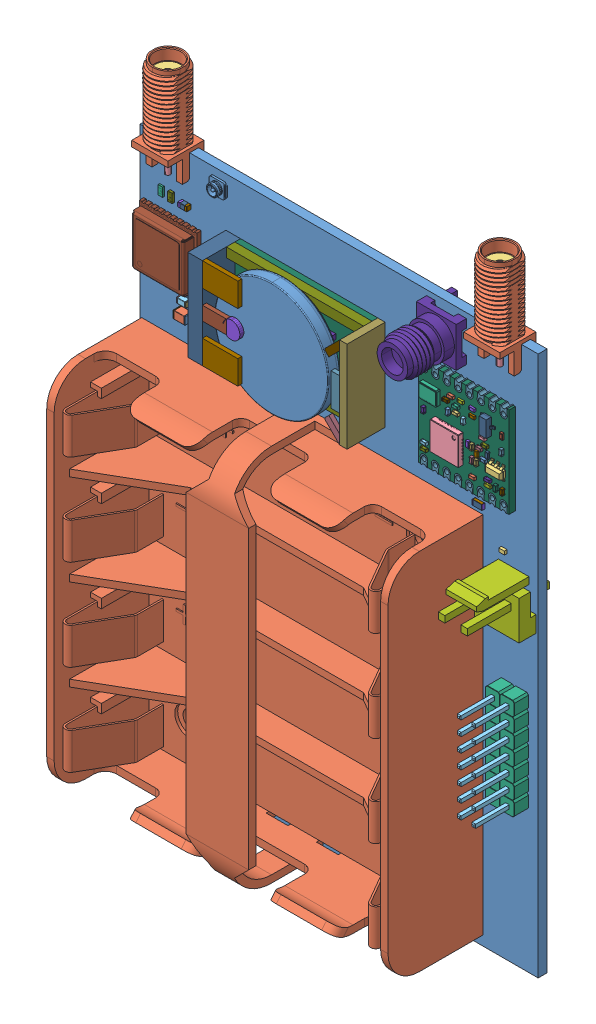
SolidWorks assembly Печатная плата Peggy Tracker, configuration Default. Lengths in mm.
Overall size (70 108.1 20.64).
358 component instances, 132 part files, 0 mates.
Components (placement in the parent):
- Печатная плата Peggy Tracker(2)^Печатная плата Peggy Tracker-1: Печатная плата Peggy Tracker(2)^Печатная плата Peggy Tracker [Default] at origin size (70 108.1 20.64) (virtual)
  - Board^Печатная плата Peggy Tracker(2)_Печатная плата Peggy Tracker-1: Board^Печатная плата Peggy Tracker(2)_Печатная плата Peggy Tracker [Default] at origin size (70 95 1.56) (virtual)
    - Open CASCADE STEP translator 6.8 1.1.1^Board_Печатная плата Peggy Tracker(2)_Печатная плата Peggy Tracker-1: Open CASCADE STEP translator 6.8 1.1.1^Board_Печатная плата Peggy Tracker(2)_Печатная плата Peggy Tracker [По умолчанию] at (0 0 -1.5596) size (70 95 1.56) (virtual)
  - XW4^Печатная плата Peggy Tracker(2)_Печатная плата Peggy Tracker-1: XW4^Печатная плата Peggy Tracker(2)_Печатная плата Peggy Tracker [Default] at origin size (6.87 17.48 6.87) (virtual)
    - SMA_female_edge_6.5x6.5^XW4_Печатная плата Peggy Tracker(2)_Печатная плата Peggy Tracker-1: SMA_female_edge_6.5x6.5^XW4_Печатная плата Peggy Tracker(2)_Печатная плата Peggy Tracker [Default] at (63.8984 92.1251 0.2) x (-1 0 0) z (0 0 1) size (6.87 17.48 6.87) (virtual)
      - SMA_female_edge_6.5x6^SMA_female_edge_6.5x6.5_XW4_Печатная плата Peggy Tracker(2)_Печатная плата Peggy Tracker-1: SMA_female_edge_6.5x6^SMA_female_edge_6.5x6.5_XW4_Печатная плата Peggy Tracker(2)_Печатная плата Peggy Tracker [Default] at origin size (6.87 17.48 6.87) (virtual)
        - ^SMA_female_edge_6.5x6_SMA_female_edge_6.5x6.5_XW4_Печатная плата Peggy Tracker(2)_Печатная плата Peggy Tracker-1: ^SMA_female_edge_6.5x6_SMA_female_edge_6.5x6.5_XW4_Печатная плата Peggy Tracker(2)_Печатная плата Peggy Tracker [По умолчанию] at (0 -4 0.45) x (0 0 1) z (0 -1 0) size (6.87 6.87 17.29) (virtual)
        - Copy (2) of ^SMA_female_edge_6.5x6_SMA_female_edge_6.5x6.5_XW4_Печатная плата Peggy Tracker(2)_Печатная плата Peggy Tracker-1: Copy (2) of ^SMA_female_edge_6.5x6_SMA_female_edge_6.5x6.5_XW4_Печатная плата Peggy Tracker(2)_Печатная плата Peggy Tracker [По умолчанию] at (0 -4 0.45) x (0 0 1) z (0 -1 0) size (4.25 4.25 11.54) (virtual)
        - Copy (3) of ^SMA_female_edge_6.5x6_SMA_female_edge_6.5x6.5_XW4_Печатная плата Peggy Tracker(2)_Печатная плата Peggy Tracker-1: Copy (3) of ^SMA_female_edge_6.5x6_SMA_female_edge_6.5x6.5_XW4_Печатная плата Peggy Tracker(2)_Печатная плата Peggy Tracker [По умолчанию] at (0 -4 0.45) x (0 0 1) z (0 -1 0) size (1.27 1.27 15.54) (virtual)
  - C21^Печатная плата Peggy Tracker(2)_Печатная плата Peggy Tracker-1: C21^Печатная плата Peggy Tracker(2)_Печатная плата Peggy Tracker [Default] at origin size (1.6 0.8 0.3) (virtual)
    - SW3dPS-0603_SMD_Capacitor^C21_Печатная плата Peggy Tracker(2)_Печатная плата Peggy Tracker-1: SW3dPS-0603_SMD_Capacitor^C21_Печатная плата Peggy Tracker(2)_Печатная плата Peggy Tracker [По умолчанию] at (25.6001 31.0999 -1.5596) x (1 0 0) z (0 1 0) size (1.6 0.3 0.8) (virtual)
  - C20^Печатная плата Peggy Tracker(2)_Печатная плата Peggy Tracker-1: C20^Печатная плата Peggy Tracker(2)_Печатная плата Peggy Tracker [Default] at origin size (3.2 1.6 1) (virtual)
    - SW3dPS-1206_SMD_Capacitor^C20_Печатная плата Peggy Tracker(2)_Печатная плата Peggy Tracker-1: SW3dPS-1206_SMD_Capacitor^C20_Печатная плата Peggy Tracker(2)_Печатная плата Peggy Tracker [По умолчанию] at (30.5 25 -1.5596) x (1 0 0) z (0 1 0) size (3.2 1 1.6) (virtual)
  - C19^Печатная плата Peggy Tracker(2)_Печатная плата Peggy Tracker-1: C19^Печатная плата Peggy Tracker(2)_Печатная плата Peggy Tracker [Default] at origin size (1.6 0.8 0.3) (virtual)
    - SW3dPS-0603_SMD_Capacitor^C19_Печатная плата Peggy Tracker(2)_Печатная плата Peggy Tracker-1: SW3dPS-0603_SMD_Capacitor^C19_Печатная плата Peggy Tracker(2)_Печатная плата Peggy Tracker [По умолчанию] at (27.9999 46.9001 -1.5596) x (-1 0 0) z (0 -1 0) size (1.6 0.3 0.8) (virtual)
  - C18^Печатная плата Peggy Tracker(2)_Печатная плата Peggy Tracker-1: C18^Печатная плата Peggy Tracker(2)_Печатная плата Peggy Tracker [Default] at origin size (0.8 1.6 0.3) (virtual)
    - SW3dPS-0603_SMD_Capacitor^C18_Печатная плата Peggy Tracker(2)_Печатная плата Peggy Tracker-1: SW3dPS-0603_SMD_Capacitor^C18_Печатная плата Peggy Tracker(2)_Печатная плата Peggy Tracker [По умолчанию] at (40.0999 43.0999 -1.5596) x (0 -1 0) z (1 0 0) size (1.6 0.3 0.8) (virtual)
  - C17^Печатная плата Peggy Tracker(2)_Печатная плата Peggy Tracker-1: C17^Печатная плата Peggy Tracker(2)_Печатная плата Peggy Tracker [Default] at origin size (0.8 1.6 0.3) (virtual)
    - SW3dPS-0603_SMD_Capacitor^C17_Печатная плата Peggy Tracker(2)_Печатная плата Peggy Tracker-1: SW3dPS-0603_SMD_Capacitor^C17_Печатная плата Peggy Tracker(2)_Печатная плата Peggy Tracker [По умолчанию] at (39.9001 34.9001 -1.5596) x (0 1 0) z (-1 0 0) size (1.6 0.3 0.8) (virtual)
  - C16^Печатная плата Peggy Tracker(2)_Печатная плата Peggy Tracker-1: C16^Печатная плата Peggy Tracker(2)_Печатная плата Peggy Tracker [Default] at origin size (1.6 0.8 0.3) (virtual)
    - SW3dPS-0603_SMD_Capacitor^C16_Печатная плата Peggy Tracker(2)_Печатная плата Peggy Tracker-1: SW3dPS-0603_SMD_Capacitor^C16_Печатная плата Peggy Tracker(2)_Печатная плата Peggy Tracker [По умолчанию] at (22.1999 32.8001 -1.5596) x (-1 0 0) z (0 -1 0) size (1.6 0.3 0.8) (virtual)
  - DD1^Печатная плата Peggy Tracker(2)_Печатная плата Peggy Tracker-1: DD1^Печатная плата Peggy Tracker(2)_Печатная плата Peggy Tracker [Default] at origin size (10.1 9.7 2.7) (virtual)
    - MAX-M8C-0^DD1_Печатная плата Peggy Tracker(2)_Печатная плата Peggy Tracker-1: MAX-M8C-0^DD1_Печатная плата Peggy Tracker(2)_Печатная плата Peggy Tracker [По умолчанию] at (5.7001 79.2999 0) x (0 1 0) z (1 0 0) size (9.7 2.7 10.1) (virtual)
  - ZQ2^Печатная плата Peggy Tracker(2)_Печатная плата Peggy Tracker-1: ZQ2^Печатная плата Peggy Tracker(2)_Печатная плата Peggy Tracker [Default] at origin size (3.22 1.52 0.91) (virtual)
    - User_Library-ABS07^ZQ2_Печатная плата Peggy Tracker(2)_Печатная плата Peggy Tracker-1: User_Library-ABS07^ZQ2_Печатная плата Peggy Tracker(2)_Печатная плата Peggy Tracker [Default] at (18.5999 54.9001 -1.5596) x (-1 0 0) z (0 -1 0) size (3.22 0.91 1.52) (virtual)
      - User_Library-ABS07_ABS07_Body_2^User_Library-ABS07_ZQ2_Печатная плата Peggy Tracker(2)_Печатная плата Peggy Tracker-1: User_Library-ABS07_ABS07_Body_2^User_Library-ABS07_ZQ2_Печатная плата Peggy Tracker(2)_Печатная плата Peggy Tracker [По умолчанию] x (1 0 0) z (0 1 0) size (3.2 1.5 0.85) (virtual)
      - User_Library-ABS07_ABS07_Body2_2^User_Library-ABS07_ZQ2_Печатная плата Peggy Tracker(2)_Печатная плата Peggy Tracker-1: User_Library-ABS07_ABS07_Body2_2^User_Library-ABS07_ZQ2_Печатная плата Peggy Tracker(2)_Печатная плата Peggy Tracker [По умолчанию] x (-1 0 0) z (0 1 0) size (3 1.3 0.05) (virtual)
      - User_Library-ABS07_ABS07_Beschriftung_2^User_Library-ABS07_ZQ2_Печатная плата Peggy Tracker(2)_Печатная плата Peggy Tracker-1: User_Library-ABS07_ABS07_Beschriftung_2^User_Library-ABS07_ZQ2_Печатная плата Peggy Tracker(2)_Печатная плата Peggy Tracker [По умолчанию] x (-1 0 0) z (0 1 0) size (2.05 0.49 0.06) (virtual)
      - User_Library-ABS07_ABS07_Pads_2^User_Library-ABS07_ZQ2_Печатная плата Peggy Tracker(2)_Печатная плата Peggy Tracker-1: User_Library-ABS07_ABS07_Pads_2^User_Library-ABS07_ZQ2_Печатная плата Peggy Tracker(2)_Печатная плата Peggy Tracker [По умолчанию] x (1 0 0) z (0 1 0) size (3.22 1.52 0.25) (virtual)
  - ZQ1^Печатная плата Peggy Tracker(2)_Печатная плата Peggy Tracker-1: ZQ1^Печатная плата Peggy Tracker(2)_Печатная плата Peggy Tracker [Default] at origin size (3.18 5 1.11) (virtual)
    - ABM3B^ZQ1_Печатная плата Peggy Tracker(2)_Печатная плата Peggy Tracker-1: ABM3B^ZQ1_Печатная плата Peggy Tracker(2)_Печатная плата Peggy Tracker [По умолчанию] at (21.4001 38.8001 -1.5596) x (0 -1 0) z (1 0 0) size (5 1.11 3.17) (virtual)
  - XW3^Печатная плата Peggy Tracker(2)_Печатная плата Peggy Tracker-1: XW3^Печатная плата Peggy Tracker(2)_Печатная плата Peggy Tracker [Default] at origin size (7.01 7.53 13.48) (virtual)
    - SMA_connector^XW3_Печатная плата Peggy Tracker(2)_Печатная плата Peggy Tracker-1: SMA_connector^XW3_Печатная плата Peggy Tracker(2)_Печатная плата Peggy Tracker [Default] at (53.9001 90.6 0) size (7.01 7.53 13.48) (virtual)
      - User_Library-SMA_Stehend_Amp_132134RP-1_1^SMA_connector_XW3_Печатная плата Peggy Tracker(2)_Печатная плата Peggy Tracker-1: User_Library-SMA_Stehend_Amp_132134RP-1_1^SMA_connector_XW3_Печатная плата Peggy Tracker(2)_Печатная плата Peggy Tracker [По умолчанию] at origin size (7.01 7.53 13.48) (virtual)
      - User_Library-SMA_Stehend_Amp_132134RP-1_2^SMA_connector_XW3_Печатная плата Peggy Tracker(2)_Печатная плата Peggy Tracker-1: User_Library-SMA_Stehend_Amp_132134RP-1_2^SMA_connector_XW3_Печатная плата Peggy Tracker(2)_Печатная плата Peggy Tracker [По умолчанию] at origin size (1.27 1.27 4.71) (virtual)
  - XW2^Печатная плата Peggy Tracker(2)_Печатная плата Peggy Tracker-1: XW2^Печатная плата Peggy Tracker(2)_Печатная плата Peggy Tracker [Default] at origin size (3.01 2.86 1.29) (virtual)
    - IPX^XW2_Печатная плата Peggy Tracker(2)_Печатная плата Peggy Tracker-1: IPX^XW2_Печатная плата Peggy Tracker(2)_Печатная плата Peggy Tracker [По умолчанию] at (13.8501 92.4001 1.27) size (3.01 2.86 1.29) (virtual)
  - XW1^Печатная плата Peggy Tracker(2)_Печатная плата Peggy Tracker-1: XW1^Печатная плата Peggy Tracker(2)_Печатная плата Peggy Tracker [Default] at origin size (6.87 17.48 6.87) (virtual)
    - SMA_female_edge_6.5x6.5^XW1_Печатная плата Peggy Tracker(2)_Печатная плата Peggy Tracker-1: SMA_female_edge_6.5x6.5^XW1_Печатная плата Peggy Tracker(2)_Печатная плата Peggy Tracker [Default] at (5.5484 92.1251 0.2) x (-1 0 0) z (0 0 1) size (6.87 17.48 6.87) (virtual)
      - SMA_female_edge_6.5x6^SMA_female_edge_6.5x6.5_XW1_Печатная плата Peggy Tracker(2)_Печатная плата Peggy Tracker-1: SMA_female_edge_6.5x6^SMA_female_edge_6.5x6.5_XW1_Печатная плата Peggy Tracker(2)_Печатная плата Peggy Tracker [Default] at origin size (6.87 17.48 6.87) (virtual)
        - ^SMA_female_edge_6.5x6_SMA_female_edge_6.5x6.5_XW1_Печатная плата Peggy Tracker(2)_Печатная плата Peggy Tracker-1: ^SMA_female_edge_6.5x6_SMA_female_edge_6.5x6.5_XW1_Печатная плата Peggy Tracker(2)_Печатная плата Peggy Tracker [По умолчанию] at (0 -4 0.45) x (0 0 1) z (0 -1 0) size (6.87 6.87 17.29) (virtual)
        - Copy (2) of ^SMA_female_edge_6.5x6_SMA_female_edge_6.5x6.5_XW1_Печатная плата Peggy Tracker(2)_Печатная плата Peggy Tracker-1: Copy (2) of ^SMA_female_edge_6.5x6_SMA_female_edge_6.5x6.5_XW1_Печатная плата Peggy Tracker(2)_Печатная плата Peggy Tracker [По умолчанию] at (0 -4 0.45) x (0 0 1) z (0 -1 0) size (4.25 4.25 11.54) (virtual)
        - Copy (3) of ^SMA_female_edge_6.5x6_SMA_female_edge_6.5x6.5_XW1_Печатная плата Peggy Tracker(2)_Печатная плата Peggy Tracker-1: Copy (3) of ^SMA_female_edge_6.5x6_SMA_female_edge_6.5x6.5_XW1_Печатная плата Peggy Tracker(2)_Печатная плата Peggy Tracker [По умолчанию] at (0 -4 0.45) x (0 0 1) z (0 -1 0) size (1.27 1.27 15.54) (virtual)
  - X5^Печатная плата Peggy Tracker(2)_Печатная плата Peggy Tracker-1: X5^Печатная плата Peggy Tracker(2)_Печатная плата Peggy Tracker [Default] at origin size (5.08 17.78 11.54) (virtual)
    - PLD-14^X5_Печатная плата Peggy Tracker(2)_Печатная плата Peggy Tracker-1: PLD-14^X5_Печатная плата Peggy Tracker(2)_Печатная плата Peggy Tracker [Default] at (64.5301 25.9799 0) x (0 -1 0) z (0 0 1) size (17.78 5.08 11.54) (virtual)
      - ____________^PLD-14_X5_Печатная плата Peggy Tracker(2)_Печатная плата Peggy Tracker-1: ____________^PLD-14_X5_Печатная плата Peggy Tracker(2)_Печатная плата Peggy Tracker [По умолчанию] at (-12.7 0 -3) size (0.64 0.64 11.54) (virtual)
      - _________^PLD-14_X5_Печатная плата Peggy Tracker(2)_Печатная плата Peggy Tracker-1: _________^PLD-14_X5_Печатная плата Peggy Tracker(2)_Печатная плата Peggy Tracker [По умолчанию] at (-5.1324 2.5342 -0.0112) size (2.54 2.54 2.54) (virtual)
      - ____________^PLD-14_X5_Печатная плата Peggy Tracker(2)_Печатная плата Peggy Tracker-2: ____________^PLD-14_X5_Печатная плата Peggy Tracker(2)_Печатная плата Peggy Tracker [По умолчанию] at (-7.62 2.54 -3) size (0.64 0.64 11.54) (virtual)
      - _________^PLD-14_X5_Печатная плата Peggy Tracker(2)_Печатная плата Peggy Tracker-2: _________^PLD-14_X5_Печатная плата Peggy Tracker(2)_Печатная плата Peggy Tracker [По умолчанию] at (-12.7524 -0.0058 -0.0112) size (2.54 2.54 2.54) (virtual)
      - ____________^PLD-14_X5_Печатная плата Peggy Tracker(2)_Печатная плата Peggy Tracker-3: ____________^PLD-14_X5_Печатная плата Peggy Tracker(2)_Печатная плата Peggy Tracker [По умолчанию] at (-15.24 2.54 -3) size (0.64 0.64 11.54) (virtual)
      - _________^PLD-14_X5_Печатная плата Peggy Tracker(2)_Печатная плата Peggy Tracker-3: _________^PLD-14_X5_Печатная плата Peggy Tracker(2)_Печатная плата Peggy Tracker [По умолчанию] at (-10.2124 2.5342 -0.0112) size (2.54 2.54 2.54) (virtual)
      - ____________^PLD-14_X5_Печатная плата Peggy Tracker(2)_Печатная плата Peggy Tracker-4: ____________^PLD-14_X5_Печатная плата Peggy Tracker(2)_Печатная плата Peggy Tracker [По умолчанию] at (-12.7 2.54 -3) size (0.64 0.64 11.54) (virtual)
      - ____________^PLD-14_X5_Печатная плата Peggy Tracker(2)_Печатная плата Peggy Tracker-5: ____________^PLD-14_X5_Печатная плата Peggy Tracker(2)_Печатная плата Peggy Tracker [По умолчанию] at (-10.16 2.54 -3) size (0.64 0.64 11.54) (virtual)
      - ____________^PLD-14_X5_Печатная плата Peggy Tracker(2)_Печатная плата Peggy Tracker-6: ____________^PLD-14_X5_Печатная плата Peggy Tracker(2)_Печатная плата Peggy Tracker [По умолчанию] at (-15.24 0 -3) size (0.64 0.64 11.54) (virtual)
      - ____________^PLD-14_X5_Печатная плата Peggy Tracker(2)_Печатная плата Peggy Tracker-7: ____________^PLD-14_X5_Печатная плата Peggy Tracker(2)_Печатная плата Peggy Tracker [По умолчанию] at (0 2.54 -3) size (0.64 0.64 11.54) (virtual)
      - ____________^PLD-14_X5_Печатная плата Peggy Tracker(2)_Печатная плата Peggy Tracker-8: ____________^PLD-14_X5_Печатная плата Peggy Tracker(2)_Печатная плата Peggy Tracker [По умолчанию] at (-7.62 0 -3) size (0.64 0.64 11.54) (virtual)
      - _________^PLD-14_X5_Печатная плата Peggy Tracker(2)_Печатная плата Peggy Tracker-4: _________^PLD-14_X5_Печатная плата Peggy Tracker(2)_Печатная плата Peggy Tracker [По умолчанию] at (-5.1324 -0.0058 -0.0112) size (2.54 2.54 2.54) (virtual)
      - _________^PLD-14_X5_Печатная плата Peggy Tracker(2)_Печатная плата Peggy Tracker-5: _________^PLD-14_X5_Печатная плата Peggy Tracker(2)_Печатная плата Peggy Tracker [По умолчанию] at (-2.5924 -0.0058 -0.0112) size (2.54 2.54 2.54) (virtual)
      - ____________^PLD-14_X5_Печатная плата Peggy Tracker(2)_Печатная плата Peggy Tracker-9: ____________^PLD-14_X5_Печатная плата Peggy Tracker(2)_Печатная плата Peggy Tracker [По умолчанию] at (-2.54 0 -3) size (0.64 0.64 11.54) (virtual)
      - ____________^PLD-14_X5_Печатная плата Peggy Tracker(2)_Печатная плата Peggy Tracker-10: ____________^PLD-14_X5_Печатная плата Peggy Tracker(2)_Печатная плата Peggy Tracker [По умолчанию] at (-5.08 0 -3) size (0.64 0.64 11.54) (virtual)
      - _________^PLD-14_X5_Печатная плата Peggy Tracker(2)_Печатная плата Peggy Tracker-6: _________^PLD-14_X5_Печатная плата Peggy Tracker(2)_Печатная плата Peggy Tracker [По умолчанию] at (-0.0524 2.5342 -0.0112) size (2.54 2.54 2.54) (virtual)
      - _________^PLD-14_X5_Печатная плата Peggy Tracker(2)_Печатная плата Peggy Tracker-7: _________^PLD-14_X5_Печатная плата Peggy Tracker(2)_Печатная плата Peggy Tracker [По умолчанию] at (-7.6724 2.5342 -0.0112) size (2.54 2.54 2.54) (virtual)
      - ____________^PLD-14_X5_Печатная плата Peggy Tracker(2)_Печатная плата Peggy Tracker-11: ____________^PLD-14_X5_Печатная плата Peggy Tracker(2)_Печатная плата Peggy Tracker [По умолчанию] at (-5.08 2.54 -3) size (0.64 0.64 11.54) (virtual)
      - _________^PLD-14_X5_Печатная плата Peggy Tracker(2)_Печатная плата Peggy Tracker-8: _________^PLD-14_X5_Печатная плата Peggy Tracker(2)_Печатная плата Peggy Tracker [По умолчанию] at (-7.6724 -0.0058 -0.0112) size (2.54 2.54 2.54) (virtual)
      - _________^PLD-14_X5_Печатная плата Peggy Tracker(2)_Печатная плата Peggy Tracker-9: _________^PLD-14_X5_Печатная плата Peggy Tracker(2)_Печатная плата Peggy Tracker [По умолчанию] at (-15.2924 2.5342 -0.0112) size (2.54 2.54 2.54) (virtual)
      - ____________^PLD-14_X5_Печатная плата Peggy Tracker(2)_Печатная плата Peggy Tracker-12: ____________^PLD-14_X5_Печатная плата Peggy Tracker(2)_Печатная плата Peggy Tracker [По умолчанию] at (-2.54 2.54 -3) size (0.64 0.64 11.54) (virtual)
      - ____________^PLD-14_X5_Печатная плата Peggy Tracker(2)_Печатная плата Peggy Tracker-13: ____________^PLD-14_X5_Печатная плата Peggy Tracker(2)_Печатная плата Peggy Tracker [По умолчанию] at (0 0 -3) size (0.64 0.64 11.54) (virtual)
      - _________^PLD-14_X5_Печатная плата Peggy Tracker(2)_Печатная плата Peggy Tracker-10: _________^PLD-14_X5_Печатная плата Peggy Tracker(2)_Печатная плата Peggy Tracker [По умолчанию] at (-10.2124 -0.0058 -0.0112) size (2.54 2.54 2.54) (virtual)
      - _________^PLD-14_X5_Печатная плата Peggy Tracker(2)_Печатная плата Peggy Tracker-11: _________^PLD-14_X5_Печатная плата Peggy Tracker(2)_Печатная плата Peggy Tracker [По умолчанию] at (-15.2924 -0.0058 -0.0112) size (2.54 2.54 2.54) (virtual)
      - _________^PLD-14_X5_Печатная плата Peggy Tracker(2)_Печатная плата Peggy Tracker-12: _________^PLD-14_X5_Печатная плата Peggy Tracker(2)_Печатная плата Peggy Tracker [По умолчанию] at (-2.5924 2.5342 -0.0112) size (2.54 2.54 2.54) (virtual)
      - _________^PLD-14_X5_Печатная плата Peggy Tracker(2)_Печатная плата Peggy Tracker-13: _________^PLD-14_X5_Печатная плата Peggy Tracker(2)_Печатная плата Peggy Tracker [По умолчанию] at (-12.7524 2.5342 -0.0112) size (2.54 2.54 2.54) (virtual)
      - _________^PLD-14_X5_Печатная плата Peggy Tracker(2)_Печатная плата Peggy Tracker-14: _________^PLD-14_X5_Печатная плата Peggy Tracker(2)_Печатная плата Peggy Tracker [По умолчанию] at (-0.0524 -0.0058 -0.0112) size (2.54 2.54 2.54) (virtual)
      - ____________^PLD-14_X5_Печатная плата Peggy Tracker(2)_Печатная плата Peggy Tracker-14: ____________^PLD-14_X5_Печатная плата Peggy Tracker(2)_Печатная плата Peggy Tracker [По умолчанию] at (-10.16 0 -3) size (0.64 0.64 11.54) (virtual)
  - X4^Печатная плата Peggy Tracker(2)_Печатная плата Peggy Tracker-1: X4^Печатная плата Peggy Tracker(2)_Печатная плата Peggy Tracker [Default] at origin size (7.86 8.5 14.4) (virtual)
    - 1-1123723-2^X4_Печатная плата Peggy Tracker(2)_Печатная плата Peggy Tracker-1: 1-1123723-2^X4_Печатная плата Peggy Tracker(2)_Печатная плата Peggy Tracker [По умолчанию] at (65.7 57.0999 3) x (1 0 0) z (0 0 1) size (7.86 8.5 14.4) (virtual)
  - X2^Печатная плата Peggy Tracker(2)_Печатная плата Peggy Tracker-1: X2^Печатная плата Peggy Tracker(2)_Печатная плата Peggy Tracker [Default] at origin size (28 20 6.7) (virtual)
    - 6036059248^X2_Печатная плата Peggy Tracker(2)_Печатная плата Peggy Tracker-1: 6036059248^X2_Печатная плата Peggy Tracker(2)_Печатная плата Peggy Tracker [Default] at (22.75 78.4 6) size (3 3 0.7) (virtual)
      - Extruded^6036059248_X2_Печатная плата Peggy Tracker(2)_Печатная плата Peggy Tracker-1: Extruded^6036059248_X2_Печатная плата Peggy Tracker(2)_Печатная плата Peggy Tracker [По умолчанию] at origin size (3 3 0.7) (virtual)
    - 6036054288^X2_Печатная плата Peggy Tracker(2)_Печатная плата Peggy Tracker-1: 6036054288^X2_Печатная плата Peggy Tracker(2)_Печатная плата Peggy Tracker [Default] at (20.7815 72.4945 6) size (6.22 4.19 0.7) (virtual)
      - Extruded-0^6036054288_X2_Печатная плата Peggy Tracker(2)_Печатная плата Peggy Tracker-1: Extruded-0^6036054288_X2_Печатная плата Peggy Tracker(2)_Печатная плата Peggy Tracker [По умолчанию] at origin size (6.22 4.19 0.7) (virtual)
    - 6036054288^X2_Печатная плата Peggy Tracker(2)_Печатная плата Peggy Tracker-2: 6036054288^X2_Печатная плата Peggy Tracker(2)_Печатная плата Peggy Tracker [Default] at (20.7815 84.3045 6) size (6.22 4.19 0.7) (virtual)
      - Extruded-0^6036054288_X2_Печатная плата Peggy Tracker(2)_Печатная плата Peggy Tracker-1: Extruded-0^6036054288_X2_Печатная плата Peggy Tracker(2)_Печатная плата Peggy Tracker [По умолчанию] at origin size (6.22 4.19 0.7) (virtual)
    - 6036054608^X2_Печатная плата Peggy Tracker(2)_Печатная плата Peggy Tracker-1: 6036054608^X2_Печатная плата Peggy Tracker(2)_Печатная плата Peggy Tracker [Default] at (16.385 78.3995 0) size (2.57 16 6.7) (virtual)
      - Extruded-1^6036054608_X2_Печатная плата Peggy Tracker(2)_Печатная плата Peggy Tracker-1: Extruded-1^6036054608_X2_Печатная плата Peggy Tracker(2)_Печатная плата Peggy Tracker [По умолчанию] at origin size (2.57 16 6.7) (virtual)
    - 6036055008^X2_Печатная плата Peggy Tracker(2)_Печатная плата Peggy Tracker-1: 6036055008^X2_Печатная плата Peggy Tracker(2)_Печатная плата Peggy Tracker [Default] at (19.7818 78.4135 6) size (4.22 2.41 0.7) (virtual)
      - Extruded-2^6036055008_X2_Печатная плата Peggy Tracker(2)_Печатная плата Peggy Tracker-1: Extruded-2^6036055008_X2_Печатная плата Peggy Tracker(2)_Печатная плата Peggy Tracker [По умолчанию] at origin size (4.22 2.41 0.7) (virtual)
    - 6036055248^X2_Печатная плата Peggy Tracker(2)_Печатная плата Peggy Tracker-1: 6036055248^X2_Печатная плата Peggy Tracker(2)_Печатная плата Peggy Tracker [Default] at (42.4492 78.3995 0) size (1.3 16 6.7) (virtual)
      - Extruded-3^6036055248_X2_Печатная плата Peggy Tracker(2)_Печатная плата Peggy Tracker-1: Extruded-3^6036055248_X2_Печатная плата Peggy Tracker(2)_Печатная плата Peggy Tracker [По умолчанию] at origin size (1.3 16 6.7) (virtual)
    - 6036055568^X2_Печатная плата Peggy Tracker(2)_Печатная плата Peggy Tracker-1: 6036055568^X2_Печатная плата Peggy Tracker(2)_Печатная плата Peggy Tracker [Default] at (40.5305 72.1757 6) size (2.54 3.55 0.7) (virtual)
      - Extruded-4^6036055568_X2_Печатная плата Peggy Tracker(2)_Печатная плата Peggy Tracker-1: Extruded-4^6036055568_X2_Печатная плата Peggy Tracker(2)_Печатная плата Peggy Tracker [По умолчанию] at origin size (2.54 3.55 0.7) (virtual)
    - 6036055968^X2_Печатная плата Peggy Tracker(2)_Печатная плата Peggy Tracker-1: 6036055968^X2_Печатная плата Peggy Tracker(2)_Печатная плата Peggy Tracker [Default] at (41.0382 78.0825 6) size (1.52 5.71 0.7) (virtual)
      - Extruded-5^6036055968_X2_Печатная плата Peggy Tracker(2)_Печатная плата Peggy Tracker-1: Extruded-5^6036055968_X2_Печатная плата Peggy Tracker(2)_Печатная плата Peggy Tracker [По умолчанию] at origin size (1.52 5.71 0.7) (virtual)
    - 6036056288^X2_Печатная плата Peggy Tracker(2)_Печатная плата Peggy Tracker-1: 6036056288^X2_Печатная плата Peggy Tracker(2)_Печатная плата Peggy Tracker [Default] at (29.7354 78.3995 0) size (24.13 16 1) (virtual)
      - Extruded-6^6036056288_X2_Печатная плата Peggy Tracker(2)_Печатная плата Peggy Tracker-1: Extruded-6^6036056288_X2_Печатная плата Peggy Tracker(2)_Печатная плата Peggy Tracker [По умолчанию] at origin size (24.13 16 1) (virtual)
    - 6036056848^X2_Печатная плата Peggy Tracker(2)_Печатная плата Peggy Tracker-1: 6036056848^X2_Печатная плата Peggy Tracker(2)_Печатная плата Peggy Tracker [Default] at (29.735 85.575 0) size (24.13 1.65 2.5) (virtual)
      - Extruded-7^6036056848_X2_Печатная плата Peggy Tracker(2)_Печатная плата Peggy Tracker-1: Extruded-7^6036056848_X2_Печатная плата Peggy Tracker(2)_Печатная плата Peggy Tracker [По умолчанию] at origin size (24.13 1.65 2.5) (virtual)
    - 6036056848^X2_Печатная плата Peggy Tracker(2)_Печатная плата Peggy Tracker-2: 6036056848^X2_Печатная плата Peggy Tracker(2)_Печатная плата Peggy Tracker [Default] at (29.7356 71.2237 0) size (24.13 1.65 2.5) (virtual)
      - Extruded-7^6036056848_X2_Печатная плата Peggy Tracker(2)_Печатная плата Peggy Tracker-1: Extruded-7^6036056848_X2_Печатная плата Peggy Tracker(2)_Печатная плата Peggy Tracker [По умолчанию] at origin size (24.13 1.65 2.5) (virtual)
    - 6036057568^X2_Печатная плата Peggy Tracker(2)_Печатная плата Peggy Tracker-1: 6036057568^X2_Печатная плата Peggy Tracker(2)_Печатная плата Peggy Tracker [Default] at (30.6875 75.4163 0) size (9.53 0.89 2.5) (virtual)
      - Extruded-8^6036057568_X2_Печатная плата Peggy Tracker(2)_Печатная плата Peggy Tracker-1: Extruded-8^6036057568_X2_Печатная плата Peggy Tracker(2)_Печатная плата Peggy Tracker [По умолчанию] at origin size (9.53 0.89 2.5) (virtual)
    - 6036057568^X2_Печатная плата Peggy Tracker(2)_Печатная плата Peggy Tracker-2: 6036057568^X2_Печатная плата Peggy Tracker(2)_Печатная плата Peggy Tracker [Default] at (30.6875 80.8773 0) size (9.53 0.89 2.5) (virtual)
      - Extruded-8^6036057568_X2_Печатная плата Peggy Tracker(2)_Печатная плата Peggy Tracker-1: Extruded-8^6036057568_X2_Печатная плата Peggy Tracker(2)_Печатная плата Peggy Tracker [По умолчанию] at origin size (9.53 0.89 2.5) (virtual)
    - 6036057888^X2_Печатная плата Peggy Tracker(2)_Печатная плата Peggy Tracker-1: 6036057888^X2_Печатная плата Peggy Tracker(2)_Печатная плата Peggy Tracker [Default] at (40.5302 84.622 6) size (2.54 3.55 0.7) (virtual)
      - Extruded-9^6036057888_X2_Печатная плата Peggy Tracker(2)_Печатная плата Peggy Tracker-1: Extruded-9^6036057888_X2_Печатная плата Peggy Tracker(2)_Печатная плата Peggy Tracker [По умолчанию] at origin size (2.54 3.55 0.7) (virtual)
    - CircuitWorks-BATT_CR2032^X2_Печатная плата Peggy Tracker(2)_Печатная плата Peggy Tracker-1: CircuitWorks-BATT_CR2032^X2_Печатная плата Peggy Tracker(2)_Печатная плата Peggy Tracker [По умолчанию] at (29.1 78.4 6) x (1 0 0) z (0 1 0) size (20 3.2 20) (virtual)
  - X1^Печатная плата Peggy Tracker(2)_Печатная плата Peggy Tracker-1: X1^Печатная плата Peggy Tracker(2)_Печатная плата Peggy Tracker [Default] at origin size (60 66.54 19.72) (virtual)
    - BK-1279-PC8--3DModel-STEP-56544^X1_Печатная плата Peggy Tracker(2)_Печатная плата Peggy Tracker-1: BK-1279-PC8--3DModel-STEP-56544^X1_Печатная плата Peggy Tracker(2)_Печатная плата Peggy Tracker [По умолчанию] at (30.3 33.7 -3.02) x (-1 0 0) z (0 1 0) size (60 19.72 66.54) (virtual)
  - VD1^Печатная плата Peggy Tracker(2)_Печатная плата Peggy Tracker-1: VD1^Печатная плата Peggy Tracker(2)_Печатная плата Peggy Tracker [Default] at origin size (1 0.6 0.53) (virtual)
    - DESD3V3S1BL-7B^VD1_Печатная плата Peggy Tracker(2)_Печатная плата Peggy Tracker-1: DESD3V3S1BL-7B^VD1_Печатная плата Peggy Tracker(2)_Печатная плата Peggy Tracker [По умолчанию] at (64.05 62.2 0) x (1 0 0) z (0 -1 0) size (1 0.53 0.6) (virtual)
  - R9^Печатная плата Peggy Tracker(2)_Печатная плата Peggy Tracker-1: R9^Печатная плата Peggy Tracker(2)_Печатная плата Peggy Tracker [Default] at origin size (0.9 1.7 0.55) (virtual)
    - 5945467952^R9_Печатная плата Peggy Tracker(2)_Печатная плата Peggy Tracker-1: 5945467952^R9_Печатная плата Peggy Tracker(2)_Печатная плата Peggy Tracker [Default] at (35.1001 47.7001 -1.5596) x (0 1 0) z (0 0 -1) size (1.7 0.9 0.55) (virtual)
      - Terminal^5945467952_R9_Печатная плата Peggy Tracker(2)_Печатная плата Peggy Tracker-1: Terminal^5945467952_R9_Печатная плата Peggy Tracker(2)_Печатная плата Peggy Tracker [Default] at (-0.85 -0.45 0) size (0.1 0.9 0.55) (virtual)
        - Open_CASCADE_STEP_translator_6.8_15.2.1^Terminal_5945467952_R9_Печатная плата Peggy Tracker(2)_Печатная плата Peggy Tracker-1: Open_CASCADE_STEP_translator_6.8_15.2.1^Terminal_5945467952_R9_Печатная плата Peggy Tracker(2)_Печатная плата Peggy Tracker [По умолчанию] at origin size (0.1 0.9 0.55) (virtual)
      - Terminal^5945467952_R9_Печатная плата Peggy Tracker(2)_Печатная плата Peggy Tracker-2: Terminal^5945467952_R9_Печатная плата Peggy Tracker(2)_Печатная плата Peggy Tracker [Default] at (0.85 0.45 0) x (-1 0 0) z (0 0 1) size (0.1 0.9 0.55) (virtual)
        - Open_CASCADE_STEP_translator_6.8_15.2.1^Terminal_5945467952_R9_Печатная плата Peggy Tracker(2)_Печатная плата Peggy Tracker-1: Open_CASCADE_STEP_translator_6.8_15.2.1^Terminal_5945467952_R9_Печатная плата Peggy Tracker(2)_Печатная плата Peggy Tracker [По умолчанию] at origin size (0.1 0.9 0.55) (virtual)
      - Mid_Body^5945467952_R9_Печатная плата Peggy Tracker(2)_Печатная плата Peggy Tracker-1: Mid_Body^5945467952_R9_Печатная плата Peggy Tracker(2)_Печатная плата Peggy Tracker [По умолчанию] at (-0.85 -0.45 0) size (1.59 0.9 0.44) (virtual)
      - Mark^5945467952_R9_Печатная плата Peggy Tracker(2)_Печатная плата Peggy Tracker-1: Mark^5945467952_R9_Печатная плата Peggy Tracker(2)_Печатная плата Peggy Tracker [По умолчанию] at (-0.75 -0.45 0.495) size (1.5 0.9 0.06) (virtual)
  - R8^Печатная плата Peggy Tracker(2)_Печатная плата Peggy Tracker-1: R8^Печатная плата Peggy Tracker(2)_Печатная плата Peggy Tracker [Default] at origin size (0.81 1.61 0.46) (virtual)
    - chip_0603_r^R8_Печатная плата Peggy Tracker(2)_Печатная плата Peggy Tracker-1: chip_0603_r^R8_Печатная плата Peggy Tracker(2)_Печатная плата Peggy Tracker [По умолчанию] at (41.6999 34.1001 -1.7696) x (-1 0 0) z (0 0 -1) size (0.81 1.61 0.46) (virtual)
  - R7^Печатная плата Peggy Tracker(2)_Печатная плата Peggy Tracker-1: R7^Печатная плата Peggy Tracker(2)_Печатная плата Peggy Tracker [Default] at origin size (1.7 0.9 0.55) (virtual)
    - 5945464112^R7_Печатная плата Peggy Tracker(2)_Печатная плата Peggy Tracker-1: 5945464112^R7_Печатная плата Peggy Tracker(2)_Печатная плата Peggy Tracker [Default] at (59.8001 67.2001 0) size (1.7 0.9 0.55) (virtual)
      - Terminal-1^5945464112_R7_Печатная плата Peggy Tracker(2)_Печатная плата Peggy Tracker-1: Terminal-1^5945464112_R7_Печатная плата Peggy Tracker(2)_Печатная плата Peggy Tracker [Default] at (-0.85 -0.45 0) size (0.1 0.9 0.55) (virtual)
        - Open_CASCADE_STEP_translator_6.8_15.2.1-10^Terminal-1_5945464112_R7_Печатная плата Peggy Tracker(2)_Печатная плата Peggy Tracker-1: Open_CASCADE_STEP_translator_6.8_15.2.1-10^Terminal-1_5945464112_R7_Печатная плата Peggy Tracker(2)_Печатная плата Peggy Tracker [По умолчанию] at origin size (0.1 0.9 0.55) (virtual)
      - Terminal-1^5945464112_R7_Печатная плата Peggy Tracker(2)_Печатная плата Peggy Tracker-2: Terminal-1^5945464112_R7_Печатная плата Peggy Tracker(2)_Печатная плата Peggy Tracker [Default] at (0.85 0.45 0) x (-1 0 0) z (0 0 1) size (0.1 0.9 0.55) (virtual)
        - Open_CASCADE_STEP_translator_6.8_15.2.1-10^Terminal-1_5945464112_R7_Печатная плата Peggy Tracker(2)_Печатная плата Peggy Tracker-1: Open_CASCADE_STEP_translator_6.8_15.2.1-10^Terminal-1_5945464112_R7_Печатная плата Peggy Tracker(2)_Печатная плата Peggy Tracker [По умолчанию] at origin size (0.1 0.9 0.55) (virtual)
      - Mid_Body-11^5945464112_R7_Печатная плата Peggy Tracker(2)_Печатная плата Peggy Tracker-1: Mid_Body-11^5945464112_R7_Печатная плата Peggy Tracker(2)_Печатная плата Peggy Tracker [По умолчанию] at (-0.85 -0.45 0) size (1.59 0.9 0.44) (virtual)
      - Mark-12^5945464112_R7_Печатная плата Peggy Tracker(2)_Печатная плата Peggy Tracker-1: Mark-12^5945464112_R7_Печатная плата Peggy Tracker(2)_Печатная плата Peggy Tracker [По умолчанию] at (-0.75 -0.45 0.495) size (1.5 0.9 0.06) (virtual)
  - R6^Печатная плата Peggy Tracker(2)_Печатная плата Peggy Tracker-1: R6^Печатная плата Peggy Tracker(2)_Печатная плата Peggy Tracker [Default] at origin size (1.61 0.81 0.46) (virtual)
    - chip_0603_r^R6_Печатная плата Peggy Tracker(2)_Печатная плата Peggy Tracker-1: chip_0603_r^R6_Печатная плата Peggy Tracker(2)_Печатная плата Peggy Tracker [По умолчанию] at (40.2001 37.4001 -1.7696) x (0 1 0) z (0 0 -1) size (0.81 1.61 0.46) (virtual)
  - R5^Печатная плата Peggy Tracker(2)_Печатная плата Peggy Tracker-1: R5^Печатная плата Peggy Tracker(2)_Печатная плата Peggy Tracker [Default] at origin size (1.61 0.81 0.46) (virtual)
    - chip_0603_r^R5_Печатная плата Peggy Tracker(2)_Печатная плата Peggy Tracker-1: chip_0603_r^R5_Печатная плата Peggy Tracker(2)_Печатная плата Peggy Tracker [По умолчанию] at (24.8999 29.2999 -1.7696) x (0 -1 0) z (0 0 -1) size (0.81 1.61 0.46) (virtual)
  - R4^Печатная плата Peggy Tracker(2)_Печатная плата Peggy Tracker-1: R4^Печатная плата Peggy Tracker(2)_Печатная плата Peggy Tracker [Default] at origin size (1.61 0.81 0.46) (virtual)
    - chip_0603_r^R4_Печатная плата Peggy Tracker(2)_Печатная плата Peggy Tracker-1: chip_0603_r^R4_Печатная плата Peggy Tracker(2)_Печатная плата Peggy Tracker [По умолчанию] at (18.0999 22.9999 -1.7696) x (0 -1 0) z (0 0 -1) size (0.81 1.61 0.46) (virtual)
  - R3^Печатная плата Peggy Tracker(2)_Печатная плата Peggy Tracker-1: R3^Печатная плата Peggy Tracker(2)_Печатная плата Peggy Tracker [Default] at origin size (0.81 1.61 0.46) (virtual)
    - chip_0603_r^R3_Печатная плата Peggy Tracker(2)_Печатная плата Peggy Tracker-1: chip_0603_r^R3_Печатная плата Peggy Tracker(2)_Печатная плата Peggy Tracker [По умолчанию] at (20.5999 17.2001 -1.7696) x (-1 0 0) z (0 0 -1) size (0.81 1.61 0.46) (virtual)
  - R2^Печатная плата Peggy Tracker(2)_Печатная плата Peggy Tracker-1: R2^Печатная плата Peggy Tracker(2)_Печатная плата Peggy Tracker [Default] at origin size (1.61 0.81 0.46) (virtual)
    - chip_0603_r^R2_Печатная плата Peggy Tracker(2)_Печатная плата Peggy Tracker-1: chip_0603_r^R2_Печатная плата Peggy Tracker(2)_Печатная плата Peggy Tracker [По умолчанию] at (14.1999 22.9999 -1.7696) x (0 -1 0) z (0 0 -1) size (0.81 1.61 0.46) (virtual)
  - R1^Печатная плата Peggy Tracker(2)_Печатная плата Peggy Tracker-1: R1^Печатная плата Peggy Tracker(2)_Печатная плата Peggy Tracker [Default] at origin size (0.81 1.61 0.46) (virtual)
    - chip_0603_r^R1_Печатная плата Peggy Tracker(2)_Печатная плата Peggy Tracker-1: chip_0603_r^R1_Печатная плата Peggy Tracker(2)_Печатная плата Peggy Tracker [По умолчанию] at (5.675 87.7 0.21) x (-1 0 0) z (0 0 1) size (0.81 1.61 0.46) (virtual)
  - MPU1^Печатная плата Peggy Tracker(2)_Печатная плата Peggy Tracker-1: MPU1^Печатная плата Peggy Tracker(2)_Печатная плата Peggy Tracker [Default] at origin size (12 12 1.2) (virtual)
    - 5945464032^MPU1_Печатная плата Peggy Tracker(2)_Печатная плата Peggy Tracker-1: 5945464032^MPU1_Печатная плата Peggy Tracker(2)_Печатная плата Peggy Tracker [Default] at (31.9001 39.0001 -1.5596) x (0 1 0) z (0 0 -1) size (12 12 1.2) (virtual)
      - Body^5945464032_MPU1_Печатная плата Peggy Tracker(2)_Печатная плата Peggy Tracker-1: Body^5945464032_MPU1_Печатная плата Peggy Tracker(2)_Печатная плата Peggy Tracker [Default] at (-5 -5 0) size (10.01 10.01 1.15) (virtual)
        - Open_CASCADE_STEP_translator_6.8_62.2.1^Body_5945464032_MPU1_Печатная плата Peggy Tracker(2)_Печатная плата Peggy Tracker-1: Open_CASCADE_STEP_translator_6.8_62.2.1^Body_5945464032_MPU1_Печатная плата Peggy Tracker(2)_Печатная плата Peggy Tracker [По умолчанию] at origin size (10.01 10.01 1.15) (virtual)
      - Open_CASCADE_STEP_translator_6.8_62.1^5945464032_MPU1_Печатная плата Peggy Tracker(2)_Печатная плата Peggy Tracker-1: Open_CASCADE_STEP_translator_6.8_62.1^5945464032_MPU1_Печатная плата Peggy Tracker(2)_Печатная плата Peggy Tracker [По умолчанию] at (-5 -5 0.001) size (1.26 1.26 0.01) (virtual)
      - Leader^5945464032_MPU1_Печатная плата Peggy Tracker(2)_Печатная плата Peggy Tracker-1: Leader^5945464032_MPU1_Печатная плата Peggy Tracker(2)_Печатная плата Peggy Tracker [По умолчанию] at (-5 -4 0) x (-1 0 0) z (0 0 1) size (1 0.38 0.68) (virtual)
      - Leader^5945464032_MPU1_Печатная плата Peggy Tracker(2)_Печатная плата Peggy Tracker-2: Leader^5945464032_MPU1_Печатная плата Peggy Tracker(2)_Печатная плата Peggy Tracker [По умолчанию] at (-5 -3.2 0) x (-1 0 0) z (0 0 1) size (1 0.38 0.68) (virtual)
